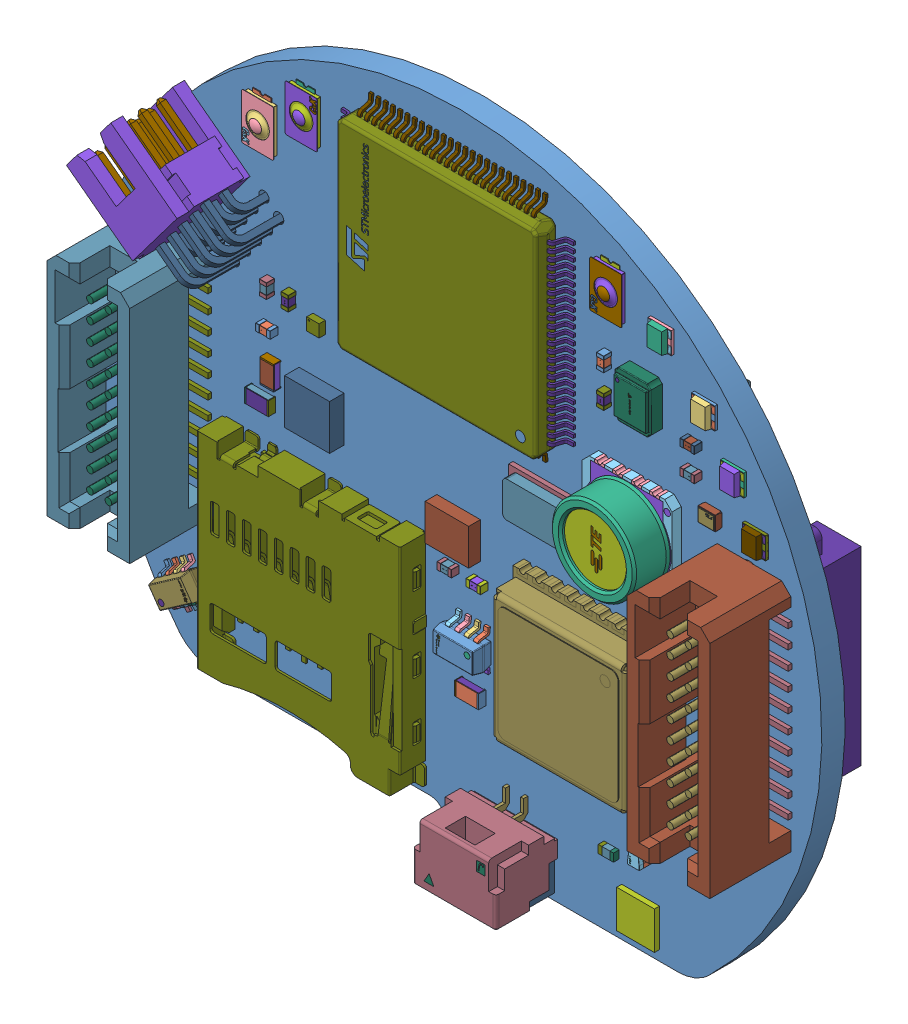
SolidWorks assembly HYDRA_V4_NAV, configuration Default. Lengths in mm. (continued)
Components (placement in the parent): (continued)
- Open CASCADE STEP translator 7.5 1024-1: Open CASCADE STEP translator 7.5 1024 [Default] at origin size (0.1 0.95 0.5)
- Open CASCADE STEP translator 7.5 1025-1: Open CASCADE STEP translator 7.5 1025 [Default] at origin size (1.45 0.95 0.05)
- Open CASCADE STEP translator 7.5 1026-1: Open CASCADE STEP translator 7.5 1026 [Default] at origin size (1.55 0.95 0.4)
- Open CASCADE STEP translator 7.5 1027-1: Open CASCADE STEP translator 7.5 1027 [Default] at origin size (0.1 0.95 0.5)
- Open CASCADE STEP translator 7.5 1028-1: Open CASCADE STEP translator 7.5 1028 [Default] at origin size (0.1 0.95 0.5)
- Open CASCADE STEP translator 7.5 1029-1: Open CASCADE STEP translator 7.5 1029 [Default] at origin size (1.45 0.95 0.05)
- Open CASCADE STEP translator 7.5 1030-1: Open CASCADE STEP translator 7.5 1030 [Default] at origin size (0.95 1.55 0.4)
- Open CASCADE STEP translator 7.5 1031-1: Open CASCADE STEP translator 7.5 1031 [Default] at origin size (0.95 0.1 0.5)
- Open CASCADE STEP translator 7.5 1032-1: Open CASCADE STEP translator 7.5 1032 [Default] at origin size (0.95 0.1 0.5)
- Open CASCADE STEP translator 7.5 1033-1: Open CASCADE STEP translator 7.5 1033 [Default] at origin size (0.95 1.45 0.05)
- Open CASCADE STEP translator 7.5 1034-1: Open CASCADE STEP translator 7.5 1034 [Default] at origin size (1.36 2.21 1.09)
- Open CASCADE STEP translator 7.5 1035-1: Open CASCADE STEP translator 7.5 1035 [Default] at origin size (0.43 0.4 0.59)
- Open CASCADE STEP translator 7.5 1036-1: Open CASCADE STEP translator 7.5 1036 [Default] at origin size (0.43 0.4 0.59)
- Open CASCADE STEP translator 7.5 1037-1: Open CASCADE STEP translator 7.5 1037 [Default] at origin size (0.43 0.4 0.59)
- Open CASCADE STEP translator 7.5 1038-1: Open CASCADE STEP translator 7.5 1038 [Default] at origin size (1.6 1.5 0.2)
- Open CASCADE STEP translator 7.5 1039-1: Open CASCADE STEP translator 7.5 1039 [Default] at origin size (1.6 1.4 0.19)
- Open CASCADE STEP translator 7.5 1040-1: Open CASCADE STEP translator 7.5 1040 [Default] at origin size (1.1 1.5 0.36)
- Open CASCADE STEP translator 7.5 1041-1: Open CASCADE STEP translator 7.5 1041 [Default] at origin size (0.5 1 0.55)
- Open CASCADE STEP translator 7.5 1042-1: Open CASCADE STEP translator 7.5 1042 [Default] at origin size (0.47 0.5 0.52)
- Open CASCADE STEP translator 7.5 1043-1: Open CASCADE STEP translator 7.5 1043 [Default] at origin size (0.03 0.3 0)
- Open CASCADE STEP translator 7.5 1044-1: Open CASCADE STEP translator 7.5 1044 [Default] at origin size (1 0.5 0.55)
- Open CASCADE STEP translator 7.5 1045-1: Open CASCADE STEP translator 7.5 1045 [Default] at origin size (0.5 0.47 0.52)
- Open CASCADE STEP translator 7.5 1046-1: Open CASCADE STEP translator 7.5 1046 [Default] at origin size (0.3 0.03 0)
- Open CASCADE STEP translator 7.5 1047-1: Open CASCADE STEP translator 7.5 1047 [Default] at origin size (0.5 1 0.55)
- Open CASCADE STEP translator 7.5 1048-1: Open CASCADE STEP translator 7.5 1048 [Default] at origin size (0.47 0.5 0.52)
- Open CASCADE STEP translator 7.5 1049-1: Open CASCADE STEP translator 7.5 1049 [Default] at origin size (0.03 0.3 0)
- Open CASCADE STEP translator 7.5 1050-1: Open CASCADE STEP translator 7.5 1050 [Default] at origin size (1 0.5 0.55)
- Open CASCADE STEP translator 7.5 1051-1: Open CASCADE STEP translator 7.5 1051 [Default] at origin size (0.5 0.47 0.52)
- Open CASCADE STEP translator 7.5 1052-1: Open CASCADE STEP translator 7.5 1052 [Default] at origin size (0.3 0.03 0)
- Open CASCADE STEP translator 7.5 1053-1: Open CASCADE STEP translator 7.5 1053 [Default] at origin size (0.5 1 0.55)
- Open CASCADE STEP translator 7.5 1054-1: Open CASCADE STEP translator 7.5 1054 [Default] at origin size (0.47 0.5 0.52)
- Open CASCADE STEP translator 7.5 1055-1: Open CASCADE STEP translator 7.5 1055 [Default] at origin size (0.03 0.3 0)
- Open CASCADE STEP translator 7.5 1056-1: Open CASCADE STEP translator 7.5 1056 [Default] at origin size (1 0.5 0.55)
- Open CASCADE STEP translator 7.5 1057-1: Open CASCADE STEP translator 7.5 1057 [Default] at origin size (0.5 0.47 0.52)
- Open CASCADE STEP translator 7.5 1058-1: Open CASCADE STEP translator 7.5 1058 [Default] at origin size (0.3 0.03 0)
- Open CASCADE STEP translator 7.5 1059-1: Open CASCADE STEP translator 7.5 1059 [Default] at origin size (0.5 1 0.55)
- Open CASCADE STEP translator 7.5 1060-1: Open CASCADE STEP translator 7.5 1060 [Default] at origin size (0.47 0.5 0.52)
- Open CASCADE STEP translator 7.5 1061-1: Open CASCADE STEP translator 7.5 1061 [Default] at origin size (0.03 0.3 0)
- Open CASCADE STEP translator 7.5 1062-1: Open CASCADE STEP translator 7.5 1062 [Default] at origin size (0.5 1 0.55)
- Open CASCADE STEP translator 7.5 1063-1: Open CASCADE STEP translator 7.5 1063 [Default] at origin size (0.47 0.5 0.52)
- Open CASCADE STEP translator 7.5 1064-1: Open CASCADE STEP translator 7.5 1064 [Default] at origin size (0.03 0.3 0)
- Open CASCADE STEP translator 7.5 1065-1: Open CASCADE STEP translator 7.5 1065 [Default] at origin size (0.5 1 0.55)
- Open CASCADE STEP translator 7.5 1066-1: Open CASCADE STEP translator 7.5 1066 [Default] at origin size (0.47 0.5 0.52)
- Open CASCADE STEP translator 7.5 1067-1: Open CASCADE STEP translator 7.5 1067 [Default] at origin size (0.03 0.3 0)
- Open CASCADE STEP translator 7.5 1068-1: Open CASCADE STEP translator 7.5 1068 [Default] at origin size (1 0.5 0.55)
- Open CASCADE STEP translator 7.5 1069-1: Open CASCADE STEP translator 7.5 1069 [Default] at origin size (0.5 0.47 0.52)
- Open CASCADE STEP translator 7.5 1070-1: Open CASCADE STEP translator 7.5 1070 [Default] at origin size (0.3 0.03 0)
- Open CASCADE STEP translator 7.5 1071-1: Open CASCADE STEP translator 7.5 1071 [Default] at origin size (0.5 1 0.55)
- Open CASCADE STEP translator 7.5 1072-1: Open CASCADE STEP translator 7.5 1072 [Default] at origin size (0.47 0.5 0.52)
- Open CASCADE STEP translator 7.5 1073-1: Open CASCADE STEP translator 7.5 1073 [Default] at origin size (0.03 0.3 0)
- Open CASCADE STEP translator 7.5 1074-1: Open CASCADE STEP translator 7.5 1074 [Default] at origin size (0.5 1 0.55)
- Open CASCADE STEP translator 7.5 1075-1: Open CASCADE STEP translator 7.5 1075 [Default] at origin size (0.47 0.5 0.52)
- Open CASCADE STEP translator 7.5 1076-1: Open CASCADE STEP translator 7.5 1076 [Default] at origin size (0.03 0.3 0)
- Open CASCADE STEP translator 7.5 1077-1: Open CASCADE STEP translator 7.5 1077 [Default] at origin size (1 0.5 0.55)
- Open CASCADE STEP translator 7.5 1078-1: Open CASCADE STEP translator 7.5 1078 [Default] at origin size (0.5 0.47 0.52)
- Open CASCADE STEP translator 7.5 1079-1: Open CASCADE STEP translator 7.5 1079 [Default] at origin size (0.3 0.03 0)
- Open CASCADE STEP translator 7.5 1080-1: Open CASCADE STEP translator 7.5 1080 [Default] at origin size (1 0.5 0.55)
- Open CASCADE STEP translator 7.5 1081-1: Open CASCADE STEP translator 7.5 1081 [Default] at origin size (0.5 0.47 0.52)
- Open CASCADE STEP translator 7.5 1082-1: Open CASCADE STEP translator 7.5 1082 [Default] at origin size (0.3 0.03 0)
- Open CASCADE STEP translator 7.5 1083-1: Open CASCADE STEP translator 7.5 1083 [Default] at origin size (1 0.5 0.55)
- Open CASCADE STEP translator 7.5 1084-1: Open CASCADE STEP translator 7.5 1084 [Default] at origin size (0.5 0.47 0.52)
- Open CASCADE STEP translator 7.5 1085-1: Open CASCADE STEP translator 7.5 1085 [Default] at origin size (0.3 0.03 0)
- Open CASCADE STEP translator 7.5 1086-1: Open CASCADE STEP translator 7.5 1086 [Default] at origin size (1 0.5 0.55)
- Open CASCADE STEP translator 7.5 1087-1: Open CASCADE STEP translator 7.5 1087 [Default] at origin size (0.5 0.47 0.52)
- Open CASCADE STEP translator 7.5 1088-1: Open CASCADE STEP translator 7.5 1088 [Default] at origin size (0.3 0.03 0)
- Open CASCADE STEP translator 7.5 1089-1: Open CASCADE STEP translator 7.5 1089 [Default] at origin size (1 0.5 0.55)
- Open CASCADE STEP translator 7.5 1090-1: Open CASCADE STEP translator 7.5 1090 [Default] at origin size (0.5 0.47 0.52)
- Open CASCADE STEP translator 7.5 1091-1: Open CASCADE STEP translator 7.5 1091 [Default] at origin size (0.3 0.03 0)
- Open CASCADE STEP translator 7.5 1092-1: Open CASCADE STEP translator 7.5 1092 [Default] at origin size (0.5 1 0.55)
- Open CASCADE STEP translator 7.5 1093-1: Open CASCADE STEP translator 7.5 1093 [Default] at origin size (0.47 0.5 0.52)
- Open CASCADE STEP translator 7.5 1094-1: Open CASCADE STEP translator 7.5 1094 [Default] at origin size (0.03 0.3 0)
- Open CASCADE STEP translator 7.5 1095-1: Open CASCADE STEP translator 7.5 1095 [Default] at origin size (1 0.5 0.55)
- Open CASCADE STEP translator 7.5 1096-1: Open CASCADE STEP translator 7.5 1096 [Default] at origin size (0.5 0.47 0.52)
- Open CASCADE STEP translator 7.5 1097-1: Open CASCADE STEP translator 7.5 1097 [Default] at origin size (0.3 0.03 0)
- Open CASCADE STEP translator 7.5 1098-1: Open CASCADE STEP translator 7.5 1098 [Default] at origin size (1 0.5 0.55)
- Open CASCADE STEP translator 7.5 1099-1: Open CASCADE STEP translator 7.5 1099 [Default] at origin size (0.5 0.47 0.52)
- Open CASCADE STEP translator 7.5 1100-1: Open CASCADE STEP translator 7.5 1100 [Default] at origin size (0.3 0.03 0)
- Open CASCADE STEP translator 7.5 1101-1: Open CASCADE STEP translator 7.5 1101 [Default] at origin size (1 0.5 0.55)
- Open CASCADE STEP translator 7.5 1102-1: Open CASCADE STEP translator 7.5 1102 [Default] at origin size (0.5 0.47 0.52)
- Open CASCADE STEP translator 7.5 1103-1: Open CASCADE STEP translator 7.5 1103 [Default] at origin size (0.3 0.03 0)
- Open CASCADE STEP translator 7.5 1104-1: Open CASCADE STEP translator 7.5 1104 [Default] at origin size (1 0.5 0.55)
- Open CASCADE STEP translator 7.5 1105-1: Open CASCADE STEP translator 7.5 1105 [Default] at origin size (0.5 0.47 0.52)
- Open CASCADE STEP translator 7.5 1106-1: Open CASCADE STEP translator 7.5 1106 [Default] at origin size (0.3 0.03 0)
- Open CASCADE STEP translator 7.5 1107-1: Open CASCADE STEP translator 7.5 1107 [Default] at origin size (1 0.5 0.55)
- Open CASCADE STEP translator 7.5 1108-1: Open CASCADE STEP translator 7.5 1108 [Default] at origin size (0.5 0.47 0.52)
- Open CASCADE STEP translator 7.5 1109-1: Open CASCADE STEP translator 7.5 1109 [Default] at origin size (0.3 0.03 0)
- Open CASCADE STEP translator 7.5 1110-1: Open CASCADE STEP translator 7.5 1110 [Default] at origin size (0.25 0.55 0.4)
- Open CASCADE STEP translator 7.5 1111-1: Open CASCADE STEP translator 7.5 1111 [Default] at origin size (0.25 0.55 0.4)
- Open CASCADE STEP translator 7.5 1112-1: Open CASCADE STEP translator 7.5 1112 [Default] at origin size (0.55 0.55 0.4)
- Open CASCADE STEP translator 7.5 1113-1: Open CASCADE STEP translator 7.5 1113 [Default] at origin size (4.71 4.67 1.1)
- Open CASCADE STEP translator 7.5 1114-1: Open CASCADE STEP translator 7.5 1114 [Default] at origin size (1.36 2.21 1.09)
- Open CASCADE STEP translator 7.5 1115-1: Open CASCADE STEP translator 7.5 1115 [Default] at origin size (0.43 0.4 0.59)
- Open CASCADE STEP translator 7.5 1116-1: Open CASCADE STEP translator 7.5 1116 [Default] at origin size (0.43 0.4 0.59)
- Open CASCADE STEP translator 7.5 1117-1: Open CASCADE STEP translator 7.5 1117 [Default] at origin size (0.43 0.4 0.59)
- Open CASCADE STEP translator 7.5 1118-1: Open CASCADE STEP translator 7.5 1118 [Default] at origin size (1.6 1.5 0.2)
- Open CASCADE STEP translator 7.5 1119-1: Open CASCADE STEP translator 7.5 1119 [Default] at origin size (1.6 1.4 0.19)
- Open CASCADE STEP translator 7.5 1120-1: Open CASCADE STEP translator 7.5 1120 [Default] at origin size (1.1 1.5 0.36)
- Open CASCADE STEP translator 7.5 1121-1: Open CASCADE STEP translator 7.5 1121 [Default] at origin size (3.01 2.01 0.76)
- Open CASCADE STEP translator 7.5 1122-1: Open CASCADE STEP translator 7.5 1122 [Default] at origin size (3 1.35 0.2)
- Open CASCADE STEP translator 7.5 1123-1: Open CASCADE STEP translator 7.5 1123 [Default] at origin size (1.29 0.37 0)
- Open CASCADE STEP translator 7.5 1124-1: Open CASCADE STEP translator 7.5 1124 [Default] at origin size (10.4 9.7 2.7)
- Open CASCADE STEP translator 7.5 1125-1: Open CASCADE STEP translator 7.5 1125 [Default] at origin size (5 3 0.3)
- Open CASCADE STEP translator 7.5 1126-1: Open CASCADE STEP translator 7.5 1126 [Default] at origin size (4.46 2.46 0.7)
- Open CASCADE STEP translator 7.5 1127-1: Open CASCADE STEP translator 7.5 1127 [Default] at origin size (4.6 4.6 1.15)
- Open CASCADE STEP translator 7.5 1128-1: Open CASCADE STEP translator 7.5 1128 [Default] at origin size (14 14 1.52)
- Open CASCADE STEP translator 7.5 1129-1: Open CASCADE STEP translator 7.5 1129 [Default] at origin size (16 12.22 0.95)
- Open CASCADE STEP translator 7.5 1130-1: Open CASCADE STEP translator 7.5 1130 [Default] at origin size (12.22 16 0.95)
- Open CASCADE STEP translator 7.5 1131-1: Open CASCADE STEP translator 7.5 1131 [Default] at origin size (12.33 12.46 0.1)
- Open CASCADE STEP translator 7.5 1132-1: Open CASCADE STEP translator 7.5 1132 [Default] at origin size (1.3 3.5 0.06)
- Open CASCADE STEP translator 7.5 1133-1: Open CASCADE STEP translator 7.5 1133 [Default] at origin size (2 3 0.57)
- Open CASCADE STEP translator 7.5 1134-1: Open CASCADE STEP translator 7.5 1134 [Default] at origin size (2.2 3.2 0.32)
- Open CASCADE STEP translator 7.5 1135-1: Open CASCADE STEP translator 7.5 1135 [Default] at origin size (0.46 0.93 0.01)
- Open CASCADE STEP translator 7.5 1136-1: Open CASCADE STEP translator 7.5 1136 [Default] at origin size (1.3 3.5 0.06)
- Open CASCADE STEP translator 7.5 1137-1: Open CASCADE STEP translator 7.5 1137 [Default] at origin size (2 3 0.57)
- Open CASCADE STEP translator 7.5 1138-1: Open CASCADE STEP translator 7.5 1138 [Default] at origin size (2.2 3.2 0.32)
- Open CASCADE STEP translator 7.5 1139-1: Open CASCADE STEP translator 7.5 1139 [Default] at origin size (0.46 0.93 0.01)
- Open CASCADE STEP translator 7.5 1140-1: Open CASCADE STEP translator 7.5 1140 [Default] at origin size (1.55 0.95 0.4)
- Open CASCADE STEP translator 7.5 1141-1: Open CASCADE STEP translator 7.5 1141 [Default] at origin size (0.1 0.95 0.5)
- Open CASCADE STEP translator 7.5 1142-1: Open CASCADE STEP translator 7.5 1142 [Default] at origin size (0.1 0.95 0.5)
- Open CASCADE STEP translator 7.5 1143-1: Open CASCADE STEP translator 7.5 1143 [Default] at origin size (1.45 0.95 0.05)
- Open CASCADE STEP translator 7.5 1144-1: Open CASCADE STEP translator 7.5 1144 [Default] at origin size (1.55 0.95 0.4)
- Open CASCADE STEP translator 7.5 1145-1: Open CASCADE STEP translator 7.5 1145 [Default] at origin size (0.1 0.95 0.5)
- Open CASCADE STEP translator 7.5 1146-1: Open CASCADE STEP translator 7.5 1146 [Default] at origin size (0.1 0.95 0.5)
- Open CASCADE STEP translator 7.5 1147-1: Open CASCADE STEP translator 7.5 1147 [Default] at origin size (1.45 0.95 0.05)
- Open CASCADE STEP translator 7.5 1148-1: Open CASCADE STEP translator 7.5 1148 [Default] at origin size (1.55 0.95 0.4)
- Open CASCADE STEP translator 7.5 1149-1: Open CASCADE STEP translator 7.5 1149 [Default] at origin size (0.1 0.95 0.5)
- Open CASCADE STEP translator 7.5 1150-1: Open CASCADE STEP translator 7.5 1150 [Default] at origin size (0.1 0.95 0.5)
- Open CASCADE STEP translator 7.5 1151-1: Open CASCADE STEP translator 7.5 1151 [Default] at origin size (1.45 0.95 0.05)
- Open CASCADE STEP translator 7.5 1152-1: Open CASCADE STEP translator 7.5 1152 [Default] at origin size (0.95 1.55 0.4)
- Open CASCADE STEP translator 7.5 1153-1: Open CASCADE STEP translator 7.5 1153 [Default] at origin size (0.95 0.1 0.5)
- Open CASCADE STEP translator 7.5 1154-1: Open CASCADE STEP translator 7.5 1154 [Default] at origin size (0.95 0.1 0.5)
- Open CASCADE STEP translator 7.5 1155-1: Open CASCADE STEP translator 7.5 1155 [Default] at origin size (0.95 1.45 0.05)
- Open CASCADE STEP translator 7.5 1156-1: Open CASCADE STEP translator 7.5 1156 [Default] at origin size (1.55 0.95 0.4)
- Open CASCADE STEP translator 7.5 1157-1: Open CASCADE STEP translator 7.5 1157 [Default] at origin size (0.1 0.95 0.5)
- Open CASCADE STEP translator 7.5 1158-1: Open CASCADE STEP translator 7.5 1158 [Default] at origin size (0.1 0.95 0.5)
- Open CASCADE STEP translator 7.5 1159-1: Open CASCADE STEP translator 7.5 1159 [Default] at origin size (1.45 0.95 0.05)
- Open CASCADE STEP translator 7.5 1160-1: Open CASCADE STEP translator 7.5 1160 [Default] at origin size (1.55 0.95 0.4)
- Open CASCADE STEP translator 7.5 1161-1: Open CASCADE STEP translator 7.5 1161 [Default] at origin size (0.1 0.95 0.5)
- Open CASCADE STEP translator 7.5 1162-1: Open CASCADE STEP translator 7.5 1162 [Default] at origin size (0.1 0.95 0.5)
- Open CASCADE STEP translator 7.5 1163-1: Open CASCADE STEP translator 7.5 1163 [Default] at origin size (1.45 0.95 0.05)
- Open CASCADE STEP translator 7.5 1164-1: Open CASCADE STEP translator 7.5 1164 [Default] at origin size (1.55 0.95 0.4)
- Open CASCADE STEP translator 7.5 1165-1: Open CASCADE STEP translator 7.5 1165 [Default] at origin size (0.1 0.95 0.5)
- Open CASCADE STEP translator 7.5 1166-1: Open CASCADE STEP translator 7.5 1166 [Default] at origin size (0.1 0.95 0.5)
- Open CASCADE STEP translator 7.5 1167-1: Open CASCADE STEP translator 7.5 1167 [Default] at origin size (1.45 0.95 0.05)
- Open CASCADE STEP translator 7.5 1168-1: Open CASCADE STEP translator 7.5 1168 [Default] at origin size (0.95 1.55 0.4)
- Open CASCADE STEP translator 7.5 1169-1: Open CASCADE STEP translator 7.5 1169 [Default] at origin size (0.95 0.1 0.5)
- Open CASCADE STEP translator 7.5 1170-1: Open CASCADE STEP translator 7.5 1170 [Default] at origin size (0.95 0.1 0.5)
- Open CASCADE STEP translator 7.5 1171-1: Open CASCADE STEP translator 7.5 1171 [Default] at origin size (0.95 1.45 0.05)
- Open CASCADE STEP translator 7.5 1172-1: Open CASCADE STEP translator 7.5 1172 [Default] at origin size (0.95 1.55 0.4)
- Open CASCADE STEP translator 7.5 1173-1: Open CASCADE STEP translator 7.5 1173 [Default] at origin size (0.95 0.1 0.5)
- Open CASCADE STEP translator 7.5 1174-1: Open CASCADE STEP translator 7.5 1174 [Default] at origin size (0.95 0.1 0.5)
- Open CASCADE STEP translator 7.5 1175-1: Open CASCADE STEP translator 7.5 1175 [Default] at origin size (0.95 1.45 0.05)
- Open CASCADE STEP translator 7.5 1176-1: Open CASCADE STEP translator 7.5 1176 [Default] at origin size (1.81 1.69 0.4)
- Open CASCADE STEP translator 7.5 1177-1: Open CASCADE STEP translator 7.5 1177 [Default] at origin size (0.65 0.82 0.5)
- Open CASCADE STEP translator 7.5 1178-1: Open CASCADE STEP translator 7.5 1178 [Default] at origin size (0.65 0.82 0.5)
- Open CASCADE STEP translator 7.5 1179-1: Open CASCADE STEP translator 7.5 1179 [Default] at origin size (1.73 1.63 0.05)
- Open CASCADE STEP translator 7.5 1180-1: Open CASCADE STEP translator 7.5 1180 [Default] at origin size (1.55 0.95 0.4)
- Open CASCADE STEP translator 7.5 1181-1: Open CASCADE STEP translator 7.5 1181 [Default] at origin size (0.1 0.95 0.5)
- Open CASCADE STEP translator 7.5 1182-1: Open CASCADE STEP translator 7.5 1182 [Default] at origin size (0.1 0.95 0.5)
- Open CASCADE STEP translator 7.5 1183-1: Open CASCADE STEP translator 7.5 1183 [Default] at origin size (1.45 0.95 0.05)
- Open CASCADE STEP translator 7.5 1184-1: Open CASCADE STEP translator 7.5 1184 [Default] at origin size (0.95 1.55 0.4)
- Open CASCADE STEP translator 7.5 1185-1: Open CASCADE STEP translator 7.5 1185 [Default] at origin size (0.95 0.1 0.5)
- Open CASCADE STEP translator 7.5 1186-1: Open CASCADE STEP translator 7.5 1186 [Default] at origin size (0.95 0.1 0.5)
- Open CASCADE STEP translator 7.5 1187-1: Open CASCADE STEP translator 7.5 1187 [Default] at origin size (0.95 1.45 0.05)
- Open CASCADE STEP translator 7.5 1188-1: Open CASCADE STEP translator 7.5 1188 [Default] at origin size (1.55 0.95 0.4)
- Open CASCADE STEP translator 7.5 1189-1: Open CASCADE STEP translator 7.5 1189 [Default] at origin size (0.1 0.95 0.5)
- Open CASCADE STEP translator 7.5 1190-1: Open CASCADE STEP translator 7.5 1190 [Default] at origin size (0.1 0.95 0.5)
- Open CASCADE STEP translator 7.5 1191-1: Open CASCADE STEP translator 7.5 1191 [Default] at origin size (1.45 0.95 0.05)
- Open CASCADE STEP translator 7.5 1192-1: Open CASCADE STEP translator 7.5 1192 [Default] at origin size (2.21 1.36 1.09)
- Open CASCADE STEP translator 7.5 1193-1: Open CASCADE STEP translator 7.5 1193 [Default] at origin size (0.4 0.43 0.59)
- Open CASCADE STEP translator 7.5 1194-1: Open CASCADE STEP translator 7.5 1194 [Default] at origin size (0.4 0.43 0.59)
- Open CASCADE STEP translator 7.5 1195-1: Open CASCADE STEP translator 7.5 1195 [Default] at origin size (0.4 0.43 0.59)
- Open CASCADE STEP translator 7.5 1196-1: Open CASCADE STEP translator 7.5 1196 [Default] at origin size (2.21 1.36 1.09)
- Open CASCADE STEP translator 7.5 1197-1: Open CASCADE STEP translator 7.5 1197 [Default] at origin size (0.4 0.43 0.59)
- Open CASCADE STEP translator 7.5 1198-1: Open CASCADE STEP translator 7.5 1198 [Default] at origin size (0.4 0.43 0.59)
- Open CASCADE STEP translator 7.5 1199-1: Open CASCADE STEP translator 7.5 1199 [Default] at origin size (0.4 0.43 0.59)
- Open CASCADE STEP translator 7.5 1200-1: Open CASCADE STEP translator 7.5 1200 [Default] at origin size (2.21 1.36 1.09)
- Open CASCADE STEP translator 7.5 1201-1: Open CASCADE STEP translator 7.5 1201 [Default] at origin size (0.4 0.43 0.59)
- Open CASCADE STEP translator 7.5 1202-1: Open CASCADE STEP translator 7.5 1202 [Default] at origin size (0.4 0.43 0.59)
- Open CASCADE STEP translator 7.5 1203-1: Open CASCADE STEP translator 7.5 1203 [Default] at origin size (0.4 0.43 0.59)
- Open CASCADE STEP translator 7.5 1204-1: Open CASCADE STEP translator 7.5 1204 [Default] at origin size (0.8 1.6 0.5)
- Open CASCADE STEP translator 7.5 1205-1: Open CASCADE STEP translator 7.5 1205 [Default] at origin size (0.75 0.77 0.6)
- Open CASCADE STEP translator 7.5 1206-1: Open CASCADE STEP translator 7.5 1206 [Default] at origin size (0.8 1.6 0.2)
- Open CASCADE STEP translator 7.5 1207-1: Open CASCADE STEP translator 7.5 1207 [Default] at origin size (0.82 1.6 0.31)
- Open CASCADE STEP translator 7.5 1208-1: Open CASCADE STEP translator 7.5 1208 [Default] at origin size (0.11 0.46 0.03)
- Open CASCADE STEP translator 7.5 1209-1: Open CASCADE STEP translator 7.5 1209 [Default] at origin size (2.6 2.6 0.35)
- Open CASCADE STEP translator 7.5 1210-1: Open CASCADE STEP translator 7.5 1210 [Default] at origin size (7.98 7.97 5.08)
- Open CASCADE STEP translator 7.5 1211-1: Open CASCADE STEP translator 7.5 1211 [Default] at origin size (6.65 6.86 1.68)
- Open CASCADE STEP translator 7.5 1212-1: Open CASCADE STEP translator 7.5 1212 [Default] at origin size (6.1 6.49 5.65)
- Open CASCADE STEP translator 7.5 1213-1: Open CASCADE STEP translator 7.5 1213 [Default] at origin size (11.95 7.6 2.76)
- Open CASCADE STEP translator 7.5 1214-1: Open CASCADE STEP translator 7.5 1214 [Default] at origin size (1.9 6.7 2.22)
- Open CASCADE STEP translator 7.5 1215-1: Open CASCADE STEP translator 7.5 1215 [Default] at origin size (6.4 5 1.77)
- Open CASCADE STEP translator 7.5 1216-1: Open CASCADE STEP translator 7.5 1216 [Default] at origin size (4.77 4.35 0.13)
- Open CASCADE STEP translator 7.5 1217-1: Open CASCADE STEP translator 7.5 1217 [Default] at origin size (1.9 6.7 2.22)
- Open CASCADE STEP translator 7.5 1218-1: Open CASCADE STEP translator 7.5 1218 [Default] at origin size (1 0.5 0.55)
- Open CASCADE STEP translator 7.5 1219-1: Open CASCADE STEP translator 7.5 1219 [Default] at origin size (0.5 0.49 0.54)
- Open CASCADE STEP translator 7.5 1220-1: Open CASCADE STEP translator 7.5 1220 [Default] at origin size (0.26 0.06 0.01)
- Open CASCADE STEP translator 7.5 1221-1: Open CASCADE STEP translator 7.5 1221 [Default] at origin size (0.5 1 0.55)
- Open CASCADE STEP translator 7.5 1222-1: Open CASCADE STEP translator 7.5 1222 [Default] at origin size (0.47 0.5 0.52)
- Open CASCADE STEP translator 7.5 1223-1: Open CASCADE STEP translator 7.5 1223 [Default] at origin size (0.03 0.3 0)
- Open CASCADE STEP translator 7.5 1224-1: Open CASCADE STEP translator 7.5 1224 [Default] at origin size (0.5 1 0.55)
- Open CASCADE STEP translator 7.5 1225-1: Open CASCADE STEP translator 7.5 1225 [Default] at origin size (0.47 0.5 0.52)
- Open CASCADE STEP translator 7.5 1226-1: Open CASCADE STEP translator 7.5 1226 [Default] at origin size (0.03 0.3 0)
- Open CASCADE STEP translator 7.5 1227-1: Open CASCADE STEP translator 7.5 1227 [Default] at origin size (1 0.5 0.55)
- Open CASCADE STEP translator 7.5 1228-1: Open CASCADE STEP translator 7.5 1228 [Default] at origin size (0.5 0.47 0.52)
- Open CASCADE STEP translator 7.5 1229-1: Open CASCADE STEP translator 7.5 1229 [Default] at origin size (0.3 0.03 0)
- Open CASCADE STEP translator 7.5 1230-1: Open CASCADE STEP translator 7.5 1230 [Default] at origin size (0.5 1 0.55)
- Open CASCADE STEP translator 7.5 1231-1: Open CASCADE STEP translator 7.5 1231 [Default] at origin size (0.47 0.5 0.52)
- Open CASCADE STEP translator 7.5 1232-1: Open CASCADE STEP translator 7.5 1232 [Default] at origin size (0.03 0.3 0)
- Open CASCADE STEP translator 7.5 1233-1: Open CASCADE STEP translator 7.5 1233 [Default] at origin size (1 0.5 0.55)
- Open CASCADE STEP translator 7.5 1234-1: Open CASCADE STEP translator 7.5 1234 [Default] at origin size (0.5 0.47 0.52)
- Open CASCADE STEP translator 7.5 1235-1: Open CASCADE STEP translator 7.5 1235 [Default] at origin size (0.3 0.03 0)
- Open CASCADE STEP translator 7.5 1236-1: Open CASCADE STEP translator 7.5 1236 [Default] at origin size (1.1 1 0.56)
- Open CASCADE STEP translator 7.5 1237-1: Open CASCADE STEP translator 7.5 1237 [Default] at origin size (0.68 0.68 0.52)
- Open CASCADE STEP translator 7.5 1238-1: Open CASCADE STEP translator 7.5 1238 [Default] at origin size (0.26 0.2 0)
- Open CASCADE STEP translator 7.5 1239-1: Open CASCADE STEP translator 7.5 1239 [Default] at origin size (1.1 1 0.56)
- Open CASCADE STEP translator 7.5 1240-1: Open CASCADE STEP translator 7.5 1240 [Default] at origin size (0.68 0.68 0.52)
- Open CASCADE STEP translator 7.5 1241-1: Open CASCADE STEP translator 7.5 1241 [Default] at origin size (0.26 0.2 0)
- Open CASCADE STEP translator 7.5 1242-1: Open CASCADE STEP translator 7.5 1242 [Default] at origin size (0.5 1 0.55)
- Open CASCADE STEP translator 7.5 1243-1: Open CASCADE STEP translator 7.5 1243 [Default] at origin size (0.47 0.5 0.52)
- Open CASCADE STEP translator 7.5 1244-1: Open CASCADE STEP translator 7.5 1244 [Default] at origin size (0.03 0.3 0)
- Open CASCADE STEP translator 7.5 1245-1: Open CASCADE STEP translator 7.5 1245 [Default] at origin size (0.5 1 0.55)
- Open CASCADE STEP translator 7.5 1246-1: Open CASCADE STEP translator 7.5 1246 [Default] at origin size (0.47 0.5 0.52)
- Open CASCADE STEP translator 7.5 1247-1: Open CASCADE STEP translator 7.5 1247 [Default] at origin size (0.03 0.3 0)
- Open CASCADE STEP translator 7.5 1248-1: Open CASCADE STEP translator 7.5 1248 [Default] at origin size (1 0.5 0.55)
- Open CASCADE STEP translator 7.5 1249-1: Open CASCADE STEP translator 7.5 1249 [Default] at origin size (0.5 0.47 0.52)
- Open CASCADE STEP translator 7.5 1250-1: Open CASCADE STEP translator 7.5 1250 [Default] at origin size (0.3 0.03 0)
- Open CASCADE STEP translator 7.5 1251-1: Open CASCADE STEP translator 7.5 1251 [Default] at origin size (1 0.5 0.55)
- Open CASCADE STEP translator 7.5 1252-1: Open CASCADE STEP translator 7.5 1252 [Default] at origin size (0.5 0.47 0.52)
- Open CASCADE STEP translator 7.5 1253-1: Open CASCADE STEP translator 7.5 1253 [Default] at origin size (0.3 0.03 0)
- Open CASCADE STEP translator 7.5 1254-1: Open CASCADE STEP translator 7.5 1254 [Default] at origin size (1 0.5 0.55)
- Open CASCADE STEP translator 7.5 1255-1: Open CASCADE STEP translator 7.5 1255 [Default] at origin size (0.5 0.47 0.52)
- Open CASCADE STEP translator 7.5 1256-1: Open CASCADE STEP translator 7.5 1256 [Default] at origin size (0.3 0.03 0)
- Open CASCADE STEP translator 7.5 1257-1: Open CASCADE STEP translator 7.5 1257 [Default] at origin size (0.5 1 0.55)
- Open CASCADE STEP translator 7.5 1258-1: Open CASCADE STEP translator 7.5 1258 [Default] at origin size (0.47 0.5 0.52)
- Open CASCADE STEP translator 7.5 1259-1: Open CASCADE STEP translator 7.5 1259 [Default] at origin size (0.03 0.3 0)
- Open CASCADE STEP translator 7.5 1260-1: Open CASCADE STEP translator 7.5 1260 [Default] at origin size (0.5 1 0.55)
- Open CASCADE STEP translator 7.5 1261-1: Open CASCADE STEP translator 7.5 1261 [Default] at origin size (0.47 0.5 0.52)
- Open CASCADE STEP translator 7.5 1262-1: Open CASCADE STEP translator 7.5 1262 [Default] at origin size (0.03 0.3 0)
- Open CASCADE STEP translator 7.5 1263-1: Open CASCADE STEP translator 7.5 1263 [Default] at origin size (0.5 1 0.55)
- Open CASCADE STEP translator 7.5 1264-1: Open CASCADE STEP translator 7.5 1264 [Default] at origin size (0.47 0.5 0.52)
- Open CASCADE STEP translator 7.5 1265-1: Open CASCADE STEP translator 7.5 1265 [Default] at origin size (0.03 0.3 0)
- Open CASCADE STEP translator 7.5 1266-1: Open CASCADE STEP translator 7.5 1266 [Default] at origin size (1 0.5 0.55)
- Open CASCADE STEP translator 7.5 1267-1: Open CASCADE STEP translator 7.5 1267 [Default] at origin size (0.5 0.47 0.52)
- Open CASCADE STEP translator 7.5 1268-1: Open CASCADE STEP translator 7.5 1268 [Default] at origin size (0.3 0.03 0)
- Open CASCADE STEP translator 7.5 1269-1: Open CASCADE STEP translator 7.5 1269 [Default] at origin size (0.5 1 0.55)
- Open CASCADE STEP translator 7.5 1270-1: Open CASCADE STEP translator 7.5 1270 [Default] at origin size (0.47 0.5 0.52)
- Open CASCADE STEP translator 7.5 1271-1: Open CASCADE STEP translator 7.5 1271 [Default] at origin size (0.03 0.3 0)
- Open CASCADE STEP translator 7.5 1272-1: Open CASCADE STEP translator 7.5 1272 [Default] at origin size (1 0.5 0.55)
- Open CASCADE STEP translator 7.5 1273-1: Open CASCADE STEP translator 7.5 1273 [Default] at origin size (0.5 0.47 0.52)
- Open CASCADE STEP translator 7.5 1274-1: Open CASCADE STEP translator 7.5 1274 [Default] at origin size (0.3 0.03 0)
- Open CASCADE STEP translator 7.5 1275-1: Open CASCADE STEP translator 7.5 1275 [Default] at origin size (1 0.5 0.55)
- Open CASCADE STEP translator 7.5 1276-1: Open CASCADE STEP translator 7.5 1276 [Default] at origin size (0.5 0.47 0.52)
- Open CASCADE STEP translator 7.5 1277-1: Open CASCADE STEP translator 7.5 1277 [Default] at origin size (0.3 0.03 0)
- Open CASCADE STEP translator 7.5 1278-1: Open CASCADE STEP translator 7.5 1278 [Default] at origin size (1 0.5 0.55)
- Open CASCADE STEP translator 7.5 1279-1: Open CASCADE STEP translator 7.5 1279 [Default] at origin size (0.5 0.47 0.52)
- Open CASCADE STEP translator 7.5 1280-1: Open CASCADE STEP translator 7.5 1280 [Default] at origin size (0.3 0.03 0)
- Open CASCADE STEP translator 7.5 1281-1: Open CASCADE STEP translator 7.5 1281 [Default] at origin size (1 0.5 0.55)
- Open CASCADE STEP translator 7.5 1282-1: Open CASCADE STEP translator 7.5 1282 [Default] at origin size (0.5 0.47 0.52)
- Open CASCADE STEP translator 7.5 1283-1: Open CASCADE STEP translator 7.5 1283 [Default] at origin size (0.3 0.03 0)
- Open CASCADE STEP translator 7.5 1284-1: Open CASCADE STEP translator 7.5 1284 [Default] at origin size (1 0.5 0.55)
- Open CASCADE STEP translator 7.5 1285-1: Open CASCADE STEP translator 7.5 1285 [Default] at origin size (0.5 0.47 0.52)
- Open CASCADE STEP translator 7.5 1286-1: Open CASCADE STEP translator 7.5 1286 [Default] at origin size (0.3 0.03 0)
- Open CASCADE STEP translator 7.5 1287-1: Open CASCADE STEP translator 7.5 1287 [Default] at origin size (0.5 1 0.55)
- Open CASCADE STEP translator 7.5 1288-1: Open CASCADE STEP translator 7.5 1288 [Default] at origin size (0.47 0.5 0.52)
- Open CASCADE STEP translator 7.5 1289-1: Open CASCADE STEP translator 7.5 1289 [Default] at origin size (0.03 0.3 0)
- Open CASCADE STEP translator 7.5 1290-1: Open CASCADE STEP translator 7.5 1290 [Default] at origin size (1 0.5 0.55)
- Open CASCADE STEP translator 7.5 1291-1: Open CASCADE STEP translator 7.5 1291 [Default] at origin size (0.5 0.47 0.52)
- Open CASCADE STEP translator 7.5 1292-1: Open CASCADE STEP translator 7.5 1292 [Default] at origin size (0.3 0.03 0)
- Open CASCADE STEP translator 7.5 1293-1: Open CASCADE STEP translator 7.5 1293 [Default] at origin size (1.6 1.5 0.2)
- Open CASCADE STEP translator 7.5 1294-1: Open CASCADE STEP translator 7.5 1294 [Default] at origin size (1.6 1.4 0.19)
- Open CASCADE STEP translator 7.5 1295-1: Open CASCADE STEP translator 7.5 1295 [Default] at origin size (1.1 1.5 0.36)
- Open CASCADE STEP translator 7.5 1296-1: Open CASCADE STEP translator 7.5 1296 [Default] at origin size (1.6 1.5 0.2)
- Open CASCADE STEP translator 7.5 1297-1: Open CASCADE STEP translator 7.5 1297 [Default] at origin size (1.6 1.4 0.19)
- Open CASCADE STEP translator 7.5 1298-1: Open CASCADE STEP translator 7.5 1298 [Default] at origin size (1.1 1.5 0.36)
- Open CASCADE STEP translator 7.5 1299-1: Open CASCADE STEP translator 7.5 1299 [Default] at origin size (1.3 3.5 0.06)
- Open CASCADE STEP translator 7.5 1300-1: Open CASCADE STEP translator 7.5 1300 [Default] at origin size (2 3 0.57)
- Open CASCADE STEP translator 7.5 1301-1: Open CASCADE STEP translator 7.5 1301 [Default] at origin size (2.2 3.2 0.32)
- Open CASCADE STEP translator 7.5 1302-1: Open CASCADE STEP translator 7.5 1302 [Default] at origin size (0.46 0.93 0.01)
- Open CASCADE STEP translator 7.5 1303-1: Open CASCADE STEP translator 7.5 1303 [Default] at origin size (5.72 15.88 6.73)
- Open CASCADE STEP translator 7.5 1304-1: Open CASCADE STEP translator 7.5 1304 [Default] at origin size (1.78 12.7 4.01)
- Open CASCADE STEP translator 7.5 1305-1: Open CASCADE STEP translator 7.5 1305 [Default] at origin size (5.84 12.7 0.83)
- Open CASCADE STEP translator 7.5 1306-1: Open CASCADE STEP translator 7.5 1306 [Default] at origin size (5.72 15.88 6.73)
- Open CASCADE STEP translator 7.5 1307-1: Open CASCADE STEP translator 7.5 1307 [Default] at origin size (1.78 12.7 4.01)
- Open CASCADE STEP translator 7.5 1308-1: Open CASCADE STEP translator 7.5 1308 [Default] at origin size (5.84 12.7 0.83)
- Open CASCADE STEP translator 7.5 1309-1: Open CASCADE STEP translator 7.5 1309 [Default] at origin size (3.68 15.88 5.84)
- Open CASCADE STEP translator 7.5 1310-1: Open CASCADE STEP translator 7.5 1310 [Default] at origin size (4.09 12.7 1.18)
- Open CASCADE STEP translator 7.5 1311-1: Open CASCADE STEP translator 7.5 1311 [Default] at origin size (3.68 15.88 5.84)
- Open CASCADE STEP translator 7.5 1312-1: Open CASCADE STEP translator 7.5 1312 [Default] at origin size (4.09 12.7 1.18)
